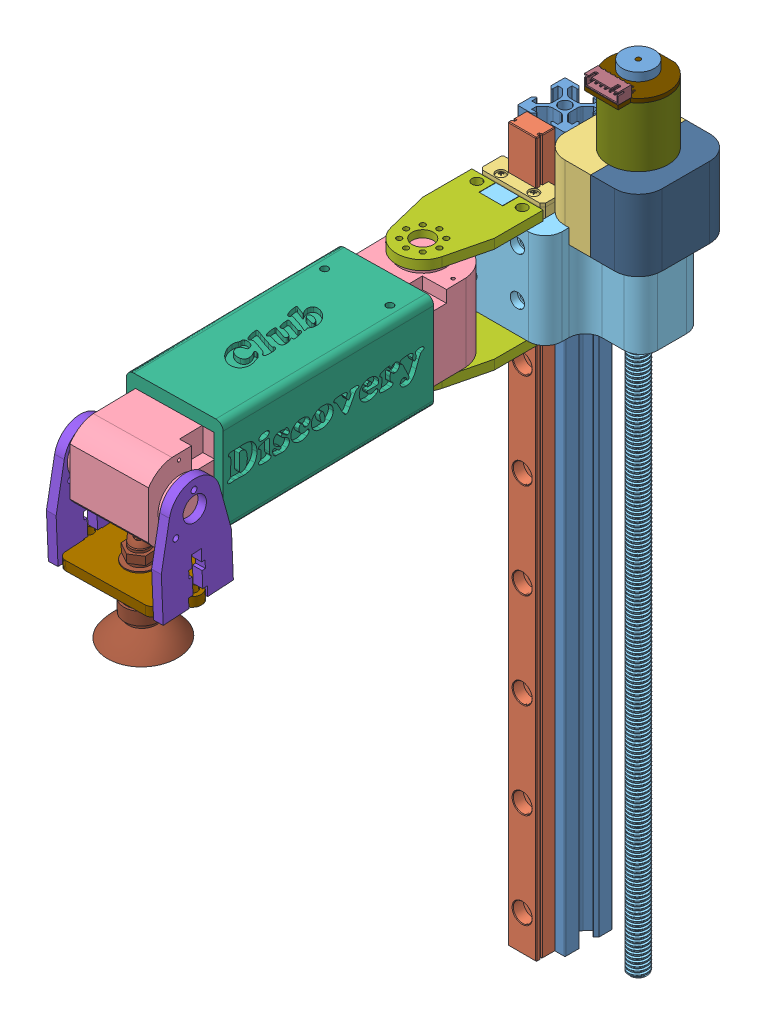
SolidWorks assembly system element de jeu vertical, configuration Default. Lengths in mm.
Overall size (75.53 333.36 220.45).
35 component instances, 29 part files, 40 mates.
Components (placement in the parent):
- FORSETI_PERFIL_20x20_V-SLOT-1: FORSETI_PERFIL_20x20_V-SLOT [Valor predeterminado] at (-26.2956 397.2794 339.6125) x (0 0 1) z (0 -1 0) size (20 20 300)
- MGN_12_H_RAIL-1: MGN_12_H_RAIL [Default] at (-20.2956 247.2794 349.6125) x (-1 0 0) z (0 1 0) size (12 8 300)
- MGN12H, LINEAR GUIDE BLOCK-1: MGN12H, LINEAR GUIDE BLOCK [Default] at (-26.2956 506.2074 355.1125) x (-1 0 0) z (0 1 0) size (27 10 47.52)
- Servo-2: Servo [Default] at (-27.2885 520.0074 407.7542) x (-0.999863 0 0.016542) z (0 -1 0) size (32 43 41.5)
- Servo-3: Servo [Default] at (-9.3369 502.7574 510.4713) x (0 -1 0) z (-0.999863 0 0.016542) size (32 43 41.5)
- tige 8 mm-1: tige 8 mm [Varsayılan] at (4.532 247.2794 339.6125) x (0.955698 0 -0.294348) z (0.294348 0 0.955698) size (8.04 264.47 9.24)
- ecrou 8mm-1: ecrou 8mm [Default] at (4.532 523.5074 339.6125) x (-0.999879 0 -0.015578) z (0 1 0) size (22 22 16.4)
- 12V 350RPM Small DFRobot Motor v8.step-1: 12V 350RPM Small DFRobot Motor v8.step [Default] at (4.532 572.2794 339.6125) x (-1 0 0) z (0 -1 0) size (25 28.09 71.15)
  - B6B-XH-AM v6.step-1: B6B-XH-AM v6.step [Default] at (0 -26 0) size (14.01 6.15 4.63)
    - Component16.step-1: Component16.step [Default] at origin size (14.01 6.15 4.63)
      - Component9.step-1: Component9.step [Default] at (5.275 15.8465 -4.0011) x (-1 0 0) z (0 0 -1) size (0.52 0.52 2.82)
      - Component12.step-1: Component12.step [Default] at (5.275 15.8465 -4.0011) x (-1 0 0) z (0 0 -1) size (0.52 0.52 2.82)
      - Component13.step-1: Component13.step [Default] at (5.275 15.8465 -4.0011) x (-1 0 0) z (0 0 -1) size (0.52 0.52 2.82)
      - Component14.step-1: Component14.step [Default] at (5.275 15.8465 -4.0011) x (-1 0 0) z (0 0 -1) size (0.52 0.52 2.82)
      - Component10.step-1: Component10.step [Default] at (5.275 15.8465 -4.0011) x (-1 0 0) z (0 0 -1) size (0.52 0.52 2.82)
      - Component11.step-1: Component11.step [Default] at (5.275 15.8465 -4.0011) x (-1 0 0) z (0 0 -1) size (0.52 0.52 2.82)
      - Main.step-1: Main.step [Default] at (5.275 16.6906 -3.9287) x (-1 0 0) z (0 -1 0) size (14.01 4.63 5.64)
  - Shaft.step-1: Shaft.step [Default] at origin size (4 4 12)
  - Shaft_Coller.step-1: Shaft_Coller.step [Default] at origin size (7 7 2.5)
  - Body_Back.step-1: Body_Back.step [Default] at origin size (25 25 31)
  - Body_Front.step-1: Body_Front.step [Default] at origin size (25 25 21)
  - PCB.step-1: PCB.step [Default] at origin size (25 27.59 7.15)
  - EncoderMagnet.step-1: EncoderMagnet.step [Default] at origin size (13.5 13.5 3.5)
  - Text.step-1: Text.step [Default] at origin size (11.44 3.52 0.02)
- support moteur 1-1: support moteur 1 [Default] at (4.532 547.2794 339.6125) x (1 0 0) z (0 -1 0) size (20.83 40 30)
- NEMA17_Coupler-1: NEMA17_Coupler [Default] at (4.532 516.2794 339.6125) x (-0.068054 0 -0.997682) z (-0.997682 0 0.068054) size (26.77 26 23.11)
- support bras 1-1: support bras 1 [Default] at (-28.952 523.5074 366.1125) x (1 0 0) z (0 -1 0) size (60.51 43.1 48)
- support servo handmade-1: support servo handmade [Default] at (-27.181 503.7574 414.2533) x (-0.999863 0 0.016542) z (0.016542 0 0.999863) size (40 45.9 90)
- support servo stock-1: support servo stock [Défaut] at (-27.4456 527.5074 369.6125) x (-1 0 0) z (0 -1 0) size (30 46.64 4)
- support servo stock-3: support servo stock [Défaut] at (-27.4456 483.5074 369.6125) x (-1 0 0) z (0 -1 0) size (30 46.64 4)
- support ventouse-3: support ventouse [Default] at (-5.7025 471.7866 518.5671) x (-0.016526 0.043392 -0.998921) z (0.999863 0 -0.016542) size (30 46 4)
- support ventouse 3-1: support ventouse 3 [Default] at (-25.4527 467.7904 518.7203) x (-0.999863 0 0.016542) z (0.000718 0.999058 0.043386) size (50.6 30 4)
- support ventouse-4: support ventouse [Default] at (-49.1965 471.7866 519.2867) x (-0.016526 0.043392 -0.998921) z (0.999863 0 -0.016542) size (30 46 4)
- support moteur 2-2: support moteur 2 [Default] at (4.532 517.2794 339.6125) x (-1 0 0) z (0 1 0) size (20 40 30)
- ventouse_final-1: ventouse_final [Default] at (-25.4703 443.2667 517.6553) x (-0.856115 -0.021808 0.516325) z (-0.516784 0.037514 -0.855293) size (30 42.25 32)
Mates (geometry in assembly coordinates):
- Coincident4: coincident aligned: plane of FORSETI_PERFIL_20x20_V-SLOT-1 through (-32.3956 547.2794 338.1086) normal (0 1 0); plane of MGN_12_H_RAIL-1 through (-32.2956 547.2794 355.6125) normal (0 1 0)
- Width14: width aligned: plane of MGN_12_H_RAIL-1 through (-32.2956 547.2794 354.8625) normal (-1 0 0); plane of MGN_12_H_RAIL-1 through (-20.2956 547.2794 354.8625) normal (1 0 0); plane of FORSETI_PERFIL_20x20_V-SLOT-1 through (-36.2956 247.2794 349.2125) normal (-1 0 0); plane of FORSETI_PERFIL_20x20_V-SLOT-1 through (-16.2956 247.2794 349.2125) normal (1 0 0)
- Coincident67: coincident anti-aligned: plane of FORSETI_PERFIL_20x20_V-SLOT-1 through (-35.8956 247.2794 349.6125) normal (0 0 1); plane of MGN_12_H_RAIL-1 through (-20.2956 547.2794 349.6125) normal (0 0 -1)
- Coincident68: coincident anti-aligned: plane of MGN_12_H_RAIL-1 through (-20.2956 547.2794 357.6125) normal (0 0 1); plane of MGN12H, LINEAR GUIDE BLOCK-1 through (-20.7956 522.4074 357.6125) normal (0 0 -1)
- LimitDistance2: limit distance = 63.772 mm anti-aligned: plane of MGN12H, LINEAR GUIDE BLOCK-1 through (-32.0456 483.5074 353.7546) normal (0 -1 0); plane of MGN_12_H_RAIL-1 through (-32.2956 547.2794 355.6125) normal (0 1 0)
- Width16: width anti-aligned: plane of MGN_12_H_RAIL-1 through (-32.2956 547.2794 354.8625) normal (-1 0 0); plane of MGN_12_H_RAIL-1 through (-20.2956 547.2794 354.8625) normal (1 0 0); plane of MGN12H, LINEAR GUIDE BLOCK-1 through (-12.7956 522.4074 362.0125) normal (1 0 0); plane of MGN12H, LINEAR GUIDE BLOCK-1 through (-39.7956 522.4074 357.4125) normal (-1 0 0)
- Concentric19: concentric anti-aligned: cylinder of 12V 350RPM Small DFRobot Motor v8.step-1/Body_Back.step-1 through (4.532 572.2794 339.6125) axis (0 -1 0) radius 12.5; cylinder of support moteur 1-1 through (4.532 517.2794 339.6125) axis (0 1 0) radius 12.5
- Parallel8: parallel aligned: plane of 12V 350RPM Small DFRobot Motor v8.step-1 through (4.532 572.2794 339.6125) normal (-1 0 0); plane of support moteur 1-1 through (-16.2956 517.2794 359.6125) normal (-1 0 0)
- Coincident73: coincident anti-aligned: plane of FORSETI_PERFIL_20x20_V-SLOT-1 through (-16.2956 247.2794 330.0125) normal (1 0 0); plane of support moteur 1-1 through (-16.2956 517.2794 359.6125) normal (-1 0 0)
- Width17: width anti-aligned: plane of support moteur 1-1 through (-16.2956 517.2794 359.6125) normal (0 0 1); plane of support moteur 1-1 through (-16.2956 517.2794 319.6125) normal (0 0 -1); plane of FORSETI_PERFIL_20x20_V-SLOT-1 through (-16.6956 247.2794 329.6125) normal (0 0 -1); plane of FORSETI_PERFIL_20x20_V-SLOT-1 through (-16.6956 247.2794 349.6125) normal (0 0 1)
- Coincident74: coincident aligned: plane of FORSETI_PERFIL_20x20_V-SLOT-1 through (-32.3956 547.2794 338.1086) normal (0 1 0); plane of support moteur 1-1 through (4.532 547.2794 339.6125) normal (0 1 0)
- Concentric21: concentric anti-aligned: cylinder of 12V 350RPM Small DFRobot Motor v8.step-1/Shaft.step-1 through (4.532 520.2794 339.6125) axis (0 -1 0) radius 2; cylinder of NEMA17_Coupler-1 through (4.532 516.2794 339.6125) axis (0 1 0) radius 2.52
- Concentric22: concentric anti-aligned: cylinder of tige 8 mm-1 through (4.532 508.7794 339.6125) axis (0 -1 0) radius 4; cylinder of NEMA17_Coupler-1 through (4.532 516.2794 339.6125) axis (0 1 0) radius 10
- Coincident76: coincident anti-aligned: plane of tige 8 mm-1 through (4.532 508.7794 339.6125) normal (0 1 0); plane of NEMA17_Coupler-1 through (4.2751 508.7794 335.8462) normal (0 -1 0)
- Concentric23: concentric anti-aligned: cylinder of tige 8 mm-1 through (4.532 508.7794 339.6125) axis (0 -1 0) radius 4; cylinder of ecrou 8mm-1 through (4.532 520.0074 339.6125) axis (0 1 0) radius 11
- Parallel9: parallel aligned: plane of FORSETI_PERFIL_20x20_V-SLOT-1 through (-32.3956 547.2794 338.1086) normal (0 1 0); plane of support bras 1-1 through (-28.952 523.5074 366.1125) normal (0 1 0)
- Coincident79: coincident aligned: plane of ecrou 8mm-1 through (4.532 523.5074 339.6125) normal (0 1 0); plane of support bras 1-1 through (-28.952 523.5074 366.1125) normal (0 1 0)
- Concentric24: concentric anti-aligned: cylinder of ecrou 8mm-1 through (4.532 520.0074 339.6125) axis (0 1 0) radius 11; cylinder of support bras 1-1 through (4.532 518.5074 339.6125) axis (0 -1 0) radius 10.8
- Coincident80: coincident aligned: plane of MGN12H, LINEAR GUIDE BLOCK-1 through (-32.0456 483.5074 353.7546) normal (0 -1 0); plane of support bras 1-1 through (-28.952 483.5074 366.1125) normal (0 -1 0)
- Parallel10: parallel anti-aligned: plane of MGN12H, LINEAR GUIDE BLOCK-1 through (-39.1956 522.4074 362.6125) normal (0 0 1); plane of support bras 1-1 through (-39.7956 483.5074 362.6125) normal (0 0 -1)
- Width19: width aligned: plane of support servo handmade-1 through (-5.6949 483.5074 503.9101) normal (0 -1 0); plane of support servo handmade-1 through (-5.6949 524.0074 503.9101) normal (0 1 0); plane of Servo-2 through (-27.2885 487.5074 407.7542) normal (0 -1 0); plane of Servo-2 through (-27.2885 520.0074 407.7542) normal (0 1 0)
- Width20: width anti-aligned: plane of Servo-3 through (-9.3369 502.7574 510.4713) normal (0.999863 0 -0.016542); plane of Servo-3 through (-41.8325 502.7574 511.0089) normal (-0.999863 0 0.016542); plane of support servo handmade-1 through (-45.6895 483.5074 504.5718) normal (-0.999863 0 0.016542); plane of support servo handmade-1 through (-5.6949 483.5074 503.9101) normal (0.999863 0 -0.016542)
- Parallel11: parallel aligned: plane of Servo-3 through (-42.1881 486.7574 489.5118) normal (0 -1 0); plane of support servo handmade-1 through (-5.6949 483.5074 503.9101) normal (0 -1 0)
- Coincident86: coincident anti-aligned: plane of support bras 1-1 through (-28.952 523.5074 366.1125) normal (0 1 0); plane of support servo stock-1 through (-27.4456 523.5074 369.6125) normal (0 -1 0)
- Coincident87: coincident anti-aligned: plane of support bras 1-1 through (-39.7956 483.5074 369.6125) normal (0 0 1); plane of support servo stock-1 through (-27.4456 523.5074 369.6125) normal (0 0 -1)
- Coincident88: coincident anti-aligned: plane of Servo-2 through (-27.4456 523.5074 398.2555) normal (0 1 0); plane of support servo stock-1 through (-27.4456 523.5074 369.6125) normal (0 -1 0)
- Width23: width aligned: plane of support servo stock-1 through (-32.4456 523.5074 369.6125) normal (1 0 0); plane of support servo stock-1 through (-22.4456 523.5074 369.6125) normal (-1 0 0); plane of support bras 1-1 through (-22.5956 527.5074 369.6125) normal (1 0 0); plane of support bras 1-1 through (-32.2956 527.5074 369.6125) normal (-1 0 0)
- Coincident90: coincident anti-aligned: plane of Servo-3 through (-41.8325 502.7574 511.0089) normal (-0.999863 0 0.016542); plane of support servo handmade-1 through (-42.1881 488.7574 489.5118) normal (0.999863 0 -0.016542)
- Coincident91: coincident anti-aligned: plane of Servo-3 through (-42.1881 518.7574 489.5118) normal (0 1 0); plane of support servo handmade-1 through (-9.6926 518.7574 488.9742) normal (0 -1 0)
- Coincident92: coincident anti-aligned: plane of Servo-3 through (-42.1881 486.7574 489.5118) normal (-0.016542 0 -0.999863); plane of support servo handmade-1 through (-25.9403 503.7574 489.243) normal (0.016542 0 0.999863)
- Concentric32: concentric aligned: cylinder of Servo-3 through (-5.6802 502.7574 519.9121) axis (-0.999863 0 0.016542) radius 9.5; cylinder of support ventouse-3 through (-1.6808 502.7574 519.8459) axis (-0.999863 0 0.016542) radius 5
- Coincident103: coincident anti-aligned: plane of Servo-3 through (-5.6802 502.7574 519.9121) normal (0.999863 0 -0.016542); plane of support ventouse-3 through (-5.7025 471.7866 518.5671) normal (-0.999863 0 0.016542)
- Coincident104: coincident anti-aligned: plane of support ventouse-3 through (-1.703 471.7866 518.5009) normal (-0.000718 -0.999058 -0.043386); plane of support ventouse 3-1 through (-25.4498 471.7866 518.8938) normal (0.000718 0.999058 0.043386)
- Width24: width anti-aligned: plane of support ventouse 3-1 through (-4.0155 471.9515 514.7423) normal (-0.016526 0.043392 -0.998921); plane of support ventouse 3-1 through (-5.8897 471.6217 522.3671) normal (0.016526 -0.043392 0.998921); plane of support ventouse-3 through (-1.7691 471.9602 514.5053) normal (0.016526 -0.043392 0.998921); plane of support ventouse-3 through (-1.6369 471.613 522.4966) normal (-0.016526 0.043392 -0.998921)
- Width25: width aligned: plane of support ventouse 3-1 through (-6.0153 471.9515 514.7753) normal (0.999863 0 -0.016542); plane of support ventouse 3-1 through (-45.0099 471.9515 515.4205) normal (-0.999863 0 0.016542); plane of support ventouse-4 through (-45.1971 471.7866 519.2205) normal (0.999863 0 -0.016542); plane of support ventouse-3 through (-5.7025 471.7866 518.5671) normal (-0.999863 0 0.016542)
- Concentric33: concentric aligned: cylinder of 12V 350RPM Small DFRobot Motor v8.step-1/Body_Back.step-1 through (4.532 572.2794 339.6125) axis (0 -1 0) radius 12.5; cylinder of support moteur 2-2 through (4.532 547.2794 339.6125) axis (0 -1 0) radius 12.5
- Coincident105: coincident anti-aligned: plane of support moteur 1-1 through (4.532 517.2794 319.6125) normal (1 0 0); plane of support moteur 2-2 through (4.532 547.2794 319.6125) normal (-1 0 0)
- Coincident106: coincident aligned: plane of support moteur 1-1 through (4.532 547.2794 339.6125) normal (0 1 0); plane of support moteur 2-2 through (4.532 547.2794 339.6125) normal (0 1 0)
- Concentric34: concentric aligned: cylinder of support ventouse 3-1 through (-25.4498 471.7866 518.8938) axis (-0.000718 -0.999058 -0.043386) radius 6.5; cylinder of ventouse_final-1 through (-25.4703 443.2667 517.6553) axis (-0.000718 -0.999058 -0.043386) radius 6.5
- Coincident107: coincident anti-aligned: plane of ventouse_final-1 through (-25.4527 467.7904 518.7203) normal (0.000718 0.999058 0.043386); plane of support ventouse 3-1 through (-25.4527 467.7904 518.7203) normal (-0.000718 -0.999058 -0.043386)
